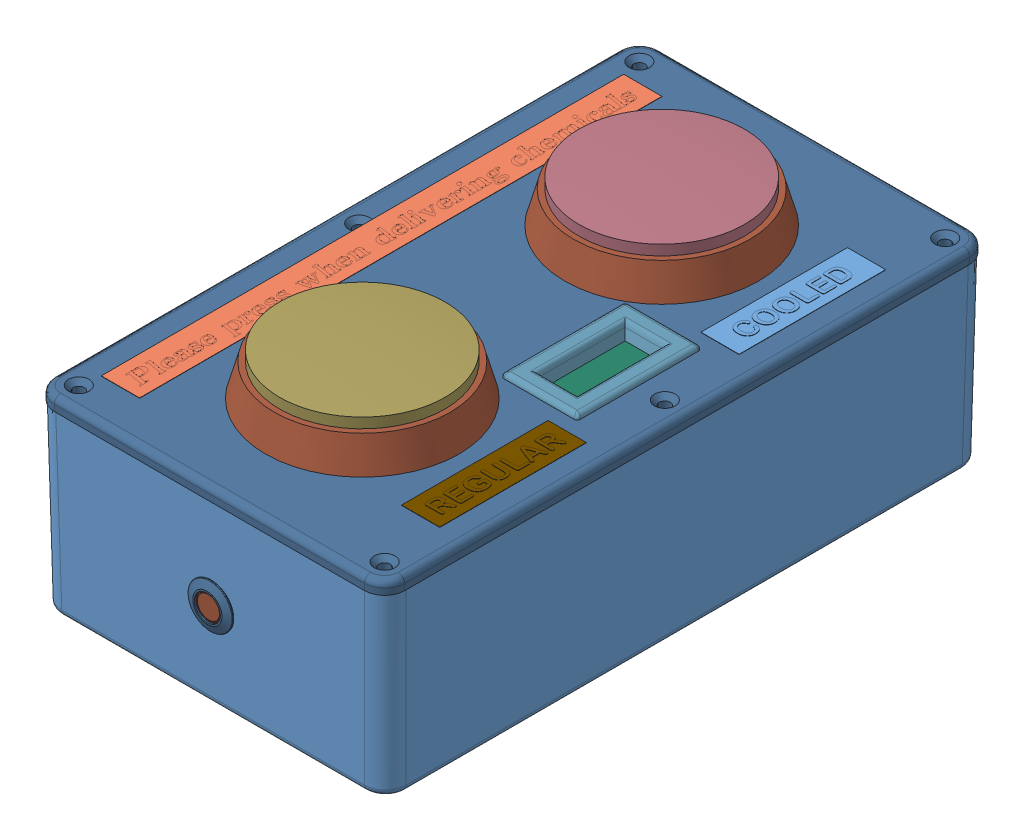
SolidWorks assembly _WiFi_Chemicals_Delivery_Bell, configuration Default. Lengths in mm.
Overall size (110 74.4 190.78).
97 component instances, 48 part files, 7 mates.
Components (placement in the parent):
- bim2006_case_bottom-1: bim2006_case_bottom [Default] at origin size (110 56 189.5)
  - bim2006_case_bottom-1: bim2006_case_bottom [Default] at (-55 -56 94.75) size (110 56 189.5)
  - insert-8: insert [Default] at (-55 -56 94.75) size (4.5 4.2 4.5)
  - insert-9: insert [Default] at (-55 -56 -81.65) size (4.5 4.2 4.5)
  - insert-10: insert [Default] at (40.5 -56 -81.65) size (4.5 4.2 4.5)
  - insert-11: insert [Default] at (40.75 -56 6.3496) size (4.5 4.2 4.5)
  - insert-12: insert [Default] at (-55.25 -56 6.3496) size (4.5 4.2 4.5)
  - insert-13: insert [Default] at (40.5 -56 94.75) size (4.5 4.2 4.5)
- circuit_board_assy-1: circuit_board_assy [Default] at (-8.473 -42.63 0) x (0 0 -1) z (1 0 0) size (51.72 30.15 47.92)
  - 2890 Doubler FeatherWing-1: 2890 Doubler FeatherWing [Default] at (-25.4 -1.57 23.5) size (50.8 1.57 47)
  - header_f12-1: header_f12 [Default] at (-10.285 0 -22.23) size (30.73 8.5 2.5)
  - header_f16-1: header_f16 [Default] at (-20.445 0 -1.91) size (40.89 8.5 2.5)
  - 2821 Adafruit ESP8266 Feather-1: 2821 Adafruit ESP8266 Feather [Default] at (-25.4 12.2142 -0.64) x (1 0 0) z (0 1 0) size (51.25 22.86 6.37)
    - 2821 Adafruit ESP8266 Feather(2)^2821 Adafruit ESP8266 Feather-1: 2821 Adafruit ESP8266 Feather(2)^2821 Adafruit ESP8266 Feather [Default] at origin size (51.25 22.86 6.37) (virtual)
      - PCB Component^2821 Adafruit ESP8266 Feather(2)_2821 Adafruit ESP8266 Feather-1: PCB Component^2821 Adafruit ESP8266 Feather(2)_2821 Adafruit ESP8266 Feather [Default] at origin size (51.25 22.86 6.37) (virtual)
        - Board^PCB Component_2821 Adafruit ESP8266 Feather(2)_2821 Adafruit ESP8266 Feather-1: Board^PCB Component_2821 Adafruit ESP8266 Feather(2)_2821 Adafruit ESP8266 Feather [Default] at origin size (50.8 22.86 1.57) (virtual)
        - 10uF^PCB Component_2821 Adafruit ESP8266 Feather(2)_2821 Adafruit ESP8266 Feather-1: 10uF^PCB Component_2821 Adafruit ESP8266 Feather(2)_2821 Adafruit ESP8266 Feather [Default] at (8.088 12.959 1.57) x (0 1 0) z (0 0 1) size (2 1.25 1) (virtual)
        - 10uF^PCB Component_2821 Adafruit ESP8266 Feather(2)_2821 Adafruit ESP8266 Feather-2: 10uF^PCB Component_2821 Adafruit ESP8266 Feather(2)_2821 Adafruit ESP8266 Feather [Default] at (14.366 12.64 1.57) x (0 -1 0) z (0 0 1) size (2 1.25 1) (virtual)
        - 10uF^PCB Component_2821 Adafruit ESP8266 Feather(2)_2821 Adafruit ESP8266 Feather-3: 10uF^PCB Component_2821 Adafruit ESP8266 Feather(2)_2821 Adafruit ESP8266 Feather [Default] at (11.049 12.192 1.57) x (-1 0 0) z (0 0 1) size (2 1.25 1) (virtual)
        - 10uF^PCB Component_2821 Adafruit ESP8266 Feather(2)_2821 Adafruit ESP8266 Feather-4: 10uF^PCB Component_2821 Adafruit ESP8266 Feather(2)_2821 Adafruit ESP8266 Feather [Default] at (21.463 16.192 1.57) x (0 -1 0) z (0 0 1) size (2 1.25 1) (virtual)
        - 10K^PCB Component_2821 Adafruit ESP8266 Feather(2)_2821 Adafruit ESP8266 Feather-1: 10K^PCB Component_2821 Adafruit ESP8266 Feather(2)_2821 Adafruit ESP8266 Feather [Default] at (12.302 4.775 1.57) x (0 -1 0) z (0 0 1) size (1.62 0.81 0.38) (virtual)
        - 10K^PCB Component_2821 Adafruit ESP8266 Feather(2)_2821 Adafruit ESP8266 Feather-2: 10K^PCB Component_2821 Adafruit ESP8266 Feather(2)_2821 Adafruit ESP8266 Feather [Default] at (6.223 4.191 1.57) size (1.62 0.81 0.38) (virtual)
        - 10K^PCB Component_2821 Adafruit ESP8266 Feather(2)_2821 Adafruit ESP8266 Feather-3: 10K^PCB Component_2821 Adafruit ESP8266 Feather(2)_2821 Adafruit ESP8266 Feather [Default] at (20.828 12.7 1.57) x (0 -1 0) z (0 0 1) size (1.62 0.81 0.38) (virtual)
        - 10K^PCB Component_2821 Adafruit ESP8266 Feather(2)_2821 Adafruit ESP8266 Feather-4: 10K^PCB Component_2821 Adafruit ESP8266 Feather(2)_2821 Adafruit ESP8266 Feather [Default] at (24.257 18.923 1.57) x (-1 0 0) z (0 0 1) size (1.62 0.81 0.38) (virtual)
        - 10K^PCB Component_2821 Adafruit ESP8266 Feather(2)_2821 Adafruit ESP8266 Feather-5: 10K^PCB Component_2821 Adafruit ESP8266 Feather(2)_2821 Adafruit ESP8266 Feather [Default] at (24.257 17.526 1.57) x (-1 0 0) z (0 0 1) size (1.62 0.81 0.38) (virtual)
        - 10K^PCB Component_2821 Adafruit ESP8266 Feather(2)_2821 Adafruit ESP8266 Feather-6: 10K^PCB Component_2821 Adafruit ESP8266 Feather(2)_2821 Adafruit ESP8266 Feather [Default] at (24.384 3.937 1.57) size (1.62 0.81 0.38) (virtual)
        - 10K^PCB Component_2821 Adafruit ESP8266 Feather(2)_2821 Adafruit ESP8266 Feather-7: 10K^PCB Component_2821 Adafruit ESP8266 Feather(2)_2821 Adafruit ESP8266 Feather [Default] at (24.384 5.334 1.57) x (-1 0 0) z (0 0 1) size (1.62 0.81 0.38) (virtual)
        - 10K^PCB Component_2821 Adafruit ESP8266 Feather(2)_2821 Adafruit ESP8266 Feather-8: 10K^PCB Component_2821 Adafruit ESP8266 Feather(2)_2821 Adafruit ESP8266 Feather [Default] at (5.588 21.082 1.57) x (0 -1 0) z (0 0 1) size (1.62 0.81 0.38) (virtual)
        - 10K^PCB Component_2821 Adafruit ESP8266 Feather(2)_2821 Adafruit ESP8266 Feather-9: 10K^PCB Component_2821 Adafruit ESP8266 Feather(2)_2821 Adafruit ESP8266 Feather [Default] at (24.003 11.938 1.57) x (-1 0 0) z (0 0 1) size (1.62 0.81 0.38) (virtual)
        - 10K^PCB Component_2821 Adafruit ESP8266 Feather(2)_2821 Adafruit ESP8266 Feather-10: 10K^PCB Component_2821 Adafruit ESP8266 Feather(2)_2821 Adafruit ESP8266 Feather [Default] at (17.78 17.272 1.57) size (1.62 0.81 0.38) (virtual)
        - MCP73831T-2ACI_OT^PCB Component_2821 Adafruit ESP8266 Feather(2)_2821 Adafruit ESP8266 Feather-1: MCP73831T-2ACI_OT^PCB Component_2821 Adafruit ESP8266 Feather(2)_2821 Adafruit ESP8266 Feather [Default] at (17.78 14.986 1.57) x (0 1 0) z (0 0 1) size (3 3 1.4) (virtual)
        - MCP73831T-2ACI_OT^PCB Component_2821 Adafruit ESP8266 Feather(2)_2821 Adafruit ESP8266 Feather-2: MCP73831T-2ACI_OT^PCB Component_2821 Adafruit ESP8266 Feather(2)_2821 Adafruit ESP8266 Feather [Default] at (17.78 11.557 1.57) x (0 -1 0) z (0 0 1) size (3 3 1.4) (virtual)
        - MBR120^PCB Component_2821 Adafruit ESP8266 Feather(2)_2821 Adafruit ESP8266 Feather-1: MBR120^PCB Component_2821 Adafruit ESP8266 Feather(2)_2821 Adafruit ESP8266 Feather [Default] at (17.907 18.796 1.57) x (-1 0 0) z (0 0 1) size (3.6 1.4 1.35) (virtual)
        - JSTPH^PCB Component_2821 Adafruit ESP8266 Feather(2)_2821 Adafruit ESP8266 Feather-1: JSTPH^PCB Component_2821 Adafruit ESP8266 Feather(2)_2821 Adafruit ESP8266 Feather [Default] at (10.795 19.304 1.57) size (7.9 8.6 4.8) (virtual)
        - RED^PCB Component_2821 Adafruit ESP8266 Feather(2)_2821 Adafruit ESP8266 Feather-1: RED^PCB Component_2821 Adafruit ESP8266 Feather(2)_2821 Adafruit ESP8266 Feather [Default] at (2.413 5.588 1.57) x (0 -1 0) z (0 0 1) size (1.25 2.02 1.1) (virtual)
        - RED^PCB Component_2821 Adafruit ESP8266 Feather(2)_2821 Adafruit ESP8266 Feather-2: RED^PCB Component_2821 Adafruit ESP8266 Feather(2)_2821 Adafruit ESP8266 Feather [Default] at (2.858 17.336 1.57) x (0 -1 0) z (0 0 1) size (1.25 2.02 1.1) (virtual)
        - ESP-12^PCB Component_2821 Adafruit ESP8266 Feather(2)_2821 Adafruit ESP8266 Feather-1: ESP-12^PCB Component_2821 Adafruit ESP8266 Feather(2)_2821 Adafruit ESP8266 Feather [Default] at (36.322 11.43 1.57) x (0 -1 0) z (0 0 1) size (16 24 2.95) (virtual)
        - KMR2^PCB Component_2821 Adafruit ESP8266 Feather(2)_2821 Adafruit ESP8266 Feather-1: KMR2^PCB Component_2821 Adafruit ESP8266 Feather(2)_2821 Adafruit ESP8266 Feather [Default] at (9.398 6.35 1.57) x (0 -1 0) z (0 0 1) size (4.6 2.8 1.94) (virtual)
        - CP2104^PCB Component_2821 Adafruit ESP8266 Feather(2)_2821 Adafruit ESP8266 Feather-1: CP2104^PCB Component_2821 Adafruit ESP8266 Feather(2)_2821 Adafruit ESP8266 Feather [Default] at (16.256 6.477 1.57) size (4 4 1) (virtual)
        - 20329^PCB Component_2821 Adafruit ESP8266 Feather(2)_2821 Adafruit ESP8266 Feather-1: 20329^PCB Component_2821 Adafruit ESP8266 Feather(2)_2821 Adafruit ESP8266 Feather [Default] at (4.445 11.43 1.57) x (0 -1 0) z (0 0 1) size (8.8 5.6 3) (virtual)
        - 1K^PCB Component_2821 Adafruit ESP8266 Feather(2)_2821 Adafruit ESP8266 Feather-1: 1K^PCB Component_2821 Adafruit ESP8266 Feather(2)_2821 Adafruit ESP8266 Feather [Default] at (24.003 10.541 1.57) size (1.6 0.9 0.8) (virtual)
        - 1K^PCB Component_2821 Adafruit ESP8266 Feather(2)_2821 Adafruit ESP8266 Feather-2: 1K^PCB Component_2821 Adafruit ESP8266 Feather(2)_2821 Adafruit ESP8266 Feather [Default] at (19.812 8.382 1.57) x (0 -1 0) z (0 0 1) size (1.6 0.9 0.8) (virtual)
        - mmbt2222^PCB Component_2821 Adafruit ESP8266 Feather(2)_2821 Adafruit ESP8266 Feather-1: mmbt2222^PCB Component_2821 Adafruit ESP8266 Feather(2)_2821 Adafruit ESP8266 Feather [Default] at (24.003 8.001 1.57) x (-1 0 0) z (0 0 1) size (3.04 2.64 1.12) (virtual)
        - mmbt2222^PCB Component_2821 Adafruit ESP8266 Feather(2)_2821 Adafruit ESP8266 Feather-2: mmbt2222^PCB Component_2821 Adafruit ESP8266 Feather(2)_2821 Adafruit ESP8266 Feather [Default] at (24.003 14.986 1.57) size (3.04 2.64 1.12) (virtual)
  - header_m16-2: header_m16 [Default] at (-20.32 9.7142 -1.91) size (40.64 11.5 2.5)
  - header_m12-1: header_m12 [Default] at (-10.16 9.7142 -22.23) size (30.48 11.5 2.5)
  - Traco TMR 1-0512-1: Traco TMR 1-0512 [Default] at (-13.58 0 19.73) size (17 15.1 7.62)
  - transistor_TO92-1: transistor_TO92 [Default] at (15.27 6 14.37) x (0 0 -1) z (1 0 0) size (5.67 13.6 4.13)
  - transistor_TO92-2: transistor_TO92 [Default] at (10.19 6 14.37) x (0 0 -1) z (1 0 0) size (5.67 13.6 4.13)
  - resistor_250mW-1: resistor_250mW [Default] at (11.4076 -3.57 6.969) size (2.5 2.5 9.06)
  - resistor_250mW-2: resistor_250mW [Default] at (6.3487 -3.57 17.1395) size (2.5 2.5 9.06)
  - header_m2-1: header_m2 [Default] at (20.32 2.5 4.45) x (-1 0 0) z (0 0 1) size (5.08 11.5 2.5)
  - header_m2-3: header_m2 [Default] at (3.81 2.5 3.18) x (0 0 1) z (1 0 0) size (5.08 11.5 2.5)
  - header_m2-4: header_m2 [Default] at (1.27 2.5 3.18) x (0 0 1) z (1 0 0) size (5.08 11.5 2.5)
  - header_m3-3: header_m3 [Default] at (-17.78 2.5 22.23) x (1 0 0) z (0 0 -1) size (7.62 11.5 2.5)
  - header_m2-5: header_m2 [Default] at (-19.05 2.5 15.88) x (0 0 1) z (1 0 0) size (5.08 11.5 2.5)
  - header_m2-6: header_m2 [Default] at (20.32 2.5 14.61) x (1 0 0) z (0 0 -1) size (5.08 11.5 2.5)
  - header_m2-7: header_m2 [Default] at (20.32 2.5 17.15) x (1 0 0) z (0 0 -1) size (5.08 11.5 2.5)
  - 3D_printed_FeatherWing_doubler_mount-1: 3D_printed_FeatherWing_doubler_mount [Default] at (0 -8.57 0) size (51.72 13 47.92)
  - ISO 4762 M2.5 x 6 - 6N-3: ISO 4762 M2.5 x 6 - 6N [ISO 4762 M2.5 x 6 - 6N] at (-22.86 2.5 -20.96) x (0 -1 0) z (0 0 1) size (8.5 4.5 4.5)
  - ISO 4762 M2.5 x 6 - 6N-2: ISO 4762 M2.5 x 6 - 6N [ISO 4762 M2.5 x 6 - 6N] at (22.86 2.5 -20.96) x (0 -1 0) z (0 0 1) size (8.5 4.5 4.5)
- bim2006_16_case_top-2: bim2006_16_case_top [Default] at origin size (110 66.8 190)
  - bim2006_16_case_top-1: bim2006_16_case_top [Default] at (-55 -56 95) size (110 6 190)
  - arcade_button_60mm_white-1: arcade_button_60mm_white [Default] at (0 4 47) x (0 0 -1) z (1 0 0) size (60.8 66.8 60.8)
    - arcade_button_60mm-1: arcade_button_60mm [Default] at origin size (60.8 62.4 60.8)
    - arcade_button_60mm_white-1: arcade_button_60mm_white [Default] at (0 10 0) size (51.9 4.4 51.9)
  - arcade_button_60mm_blue-1: arcade_button_60mm_blue [Default] at (0 4 -47) x (0 0 -1) z (1 0 0) size (60.8 66.8 60.8)
    - arcade_button_60mm-1: arcade_button_60mm [Default] at origin size (60.8 62.4 60.8)
    - arcade_button_60mm_blue-1: arcade_button_60mm_blue [Default] at (0 10 0) size (51.9 4.4 51.9)
  - 3D_printed_OLED_bezel-1: 3D_printed_OLED_bezel [Default] at (40 4 19.5) x (0 0 -1) z (1 0 0) size (39 4.23 24)
  - OLED_screen_in_tray-1: OLED_screen_in_tray [Default] at (39.62 -0.6 27.5) x (0 0 -1) z (1 0 0) size (74 11.07 30)
    - 2900 Feather OLED Wing-1: 2900 Feather OLED Wing [Default] x (1 0 0) z (0 1 0) size (50.8 22.86 6)
    - 3D_printed_OLED_tray_part_1-1: 3D_printed_OLED_tray_part_1 [Default] at (25.4 2.8 -11.43) size (74 8.57 30)
    - ISO 4762 M2.5 x 6 - 6N-3: ISO 4762 M2.5 x 6 - 6N [ISO 4762 M2.5 x 6 - 6N] at (2.54 2.5 -20.32) x (0 -1 0) z (0.175451 0 -0.984488) size (8.5 4.5 4.5)
    - 3D_printed_OLED_tray_part_2-1: 3D_printed_OLED_tray_part_2 [Default] at (-7.6 -2.6 -11.43) size (7 5.57 30)
    - ISO 4762 M2.5 x 6 - 6N-2: ISO 4762 M2.5 x 6 - 6N [ISO 4762 M2.5 x 6 - 6N] at (-7.6 -8.1 -0.43) x (0 1 0) z (0 0 1) size (8.5 4.5 4.5)
    - ISO 4762 M2.5 x 6 - 6N-4: ISO 4762 M2.5 x 6 - 6N [ISO 4762 M2.5 x 6 - 6N] at (58.4 -8.1 -0.43) x (0 1 0) z (0 0 -1) size (8.5 4.5 4.5)
    - 3D_printed_OLED_tray_part_2-2: 3D_printed_OLED_tray_part_2 [Default] at (58.4 -2.6 -11.43) size (7 5.57 30)
  - label_REGULAR-1: label_REGULAR [Default] at (47.3155 4.1 70) x (0 0 -1) z (1 0 0) size (46 0.2 12)
  - label_COOLED-1: label_COOLED [Default] at (47.3155 4.1 -24) x (0 0 -1) z (1 0 0) size (46 0.2 12)
  - label_header-1: label_header [Default] at (-34.9399 4.1 82) x (0 0 -1) z (1 0 0) size (164 0.1 12)
- 3258 microUSB panel mount-1: 3258 microUSB panel mount [Default] at (-31.1433 -43.4995 92.95) size (25 9.8 30.8)
- 12mm flat Round head Waterproof Momentary Latching Metal Push Button Switch v11-1: 12mm flat Round head Waterproof Momentary Latching Metal Push Button Switch v11 [Default] at (0 -28.6761 94.2495) x (1 0 0) z (0 -0.017452 0.999848) size (15.79 14.76 24.73)
  - 12mm flat Round head Waterproof Momentary Latching Metal Push Button Switch v11.step-1: 12mm flat Round head Waterproof Momentary Latching Metal Push Button Switch v11.step [Default] at origin size (15.79 14.76 24.73)
    - latching.step-1: latching.step [Default] at (0 0 -14.24) x (-1 0 0) z (0 0 -1) size (9.36 10.92 9.09)
      - solderlug.step-1: solderlug.step [Default] at origin size (2 0.5 4.09)
      - solderlug.step-2: solderlug.step [Default] x (0 1 0) z (0 0 1) size (2 0.5 4.09)
      - solderlug.step-3: solderlug.step [Default] x (-1 0 0) z (0 0 1) size (2 0.5 4.09)
      - solderlug.step-4: solderlug.step [Default] x (0 -1 0) z (0 0 1) size (2 0.5 4.09)
      - latching-0.step-1: latching-0.step [Default] at origin size (5.3 0.69 5)
      - latching-1.step-1: latching-1.step [Default] at origin size (2.03 9.53 5)
      - latching-2.step-1: latching-2.step [Default] at origin size (2.03 9.53 5)
      - latching-3.step-1: latching-3.step [Default] at origin size (5.3 0.69 5)
      - latching-4.step-1: latching-4.step [Default] at origin size (5.1 9.35 5.1)
    - Body.step-1: Body.step [Default] at origin size (14 14 15.64)
    - button.step-1: button.step [Default] at (0 0 -0.2414) size (8.06 8.06 1)
    - Nut.step-1: Nut.step [Default] at (0 0 -5.8) size (15.79 14.76 2.3)
Mates (geometry in assembly coordinates):
- Coincident19: coincident anti-aligned: plane of bim2006_26_case_bottom-1/bim2006_26_case_bottom-1 through (-55 0 -94.75) normal (0 1 0); plane of bim2006_16_case_top-2/bim2006_16_case_top-1 through (-48.7 0 -88.7) normal (0 -1 0)
- Coincident20: coincident aligned: plane of bim2006_26_case_bottom-1 through (0 0 0) normal (1 0 0); plane of bim2006_16_case_top-2/bim2006_16_case_top-1 through (0 -56 95) normal (1 0 0)
- Distance1: distance = 1 mm anti-aligned: plane of bim2006_case_bottom-1/bim2006_case_bottom-1 through (-36.45 3.2651 91.95) normal (0 0 -1); plane of 3258 microUSB panel mount-1 through (-31.1433 -43.4995 92.95) normal (0 0 1)
- Coincident23: coincident aligned: plane of bim2006_case_bottom-1 through (0 0 0) normal (0 0 1); plane of circuit_board_assy-1/2890 Doubler FeatherWing-1 through (15.027 -44.2 0) normal (0 0 1)
- Coincident27: coincident anti-aligned: plane of bim2006_case_bottom-1/bim2006_case_bottom-1 through (-53.2 -54.2 -92.95) normal (0 1 0); plane of circuit_board_assy-1/3D_printed_FeatherWing_doubler_mount-1 through (-29.433 -54.2 22.86) normal (0 -1 0)
- Coincident28: coincident anti-aligned: plane of bim2006_case_bottom-1/bim2006_case_bottom-1 through (-55 0 94.75) normal (0 -0.017452 0.999848); plane of 12mm flat Round head Waterproof Momentary Latching Metal Push Button Switch v11-1/12mm flat Round head Waterproof Momentary Latching Metal Push Button Switch v11.step-1/Body.step-1 through (7 -28.6761 94.2495) normal (0 0.017452 -0.999848)
- Coincident29: coincident aligned: plane of bim2006_case_bottom-1 through (0 0 0) normal (1 0 0); plane of 12mm flat Round head Waterproof Momentary Latching Metal Push Button Switch v11-1 through (0 -28.6761 94.2495) normal (1 0 0)
